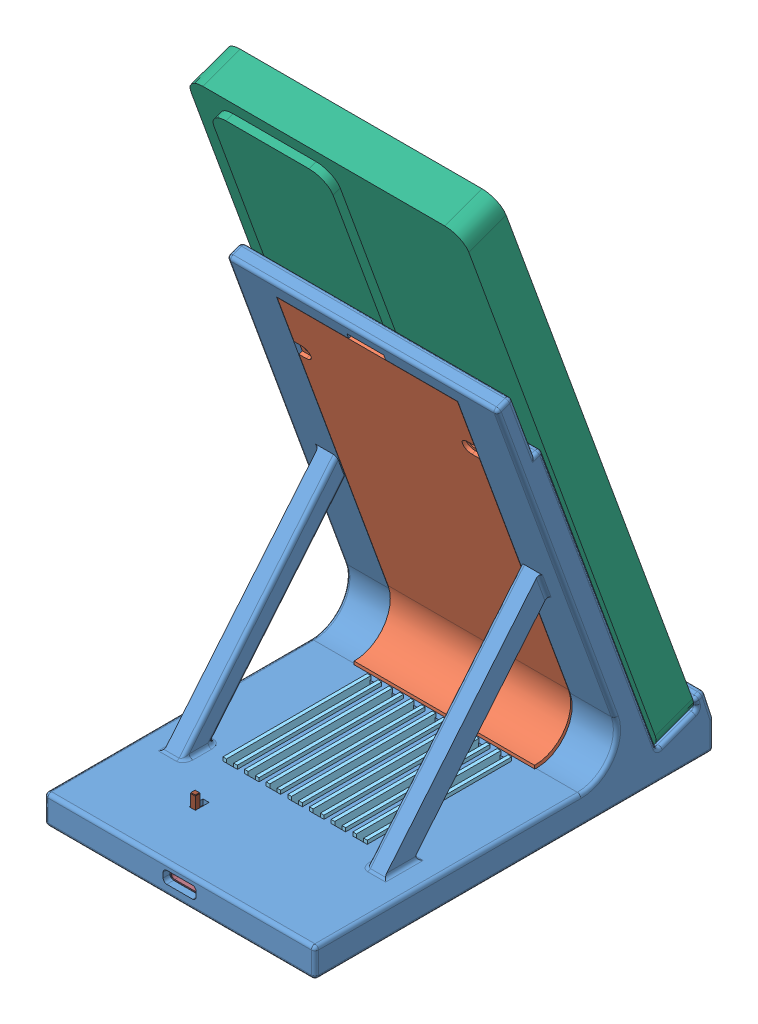
SolidWorks assembly IP支架装配体_倒, configuration 默认. Lengths in mm.
Overall size (77 163.11 111.5).
38 component instances, 18 part files, 24 mates.
Components (placement in the parent):
- IP支架_倒-1: IP支架_倒 [默认] at (-67.6479 -61.183 124.564) size (75 112.62 110.5)
- 支架零件-1: 支架零件 [默认] at (-67.6479 -57.3497 135.0646) x (0 0 -1) z (1 0 0) size (34.38 102 50)
- IP手机-1: IP手机 [默认] at (-19.3867 44.2514 95.8225) x (1 0 0) z (0 0.939693 0.34202) size (76 12 151) (hidden)
- 充电线圈-1: 充电线圈 [默认] at (-67.6479 22.7276 116.3435) x (1 0 0) z (0 -0.939693 -0.34202) size (43 1.52 55.03)
- 充电零件板-1: 充电零件板 [默认] at (-67.7479 -57.183 127.464) x (1 0 0) z (0 0 -1) size (21 2 28)
- 散热器-1: 散热器 [默认] at (-67.7479 -57.183 127.464) size (40 5 40)
- P60手机-1: P60手机 [默认] at (-67.6479 22.4622 112.0966) x (-1 0 0) z (0 0.34202 -0.939693) size (77 161 13.1)
- Led5mmRojo_.step-1: Led5mmRojo_.step [默认] at (-67.6479 -56.683 93.564) x (0 0 -1) z (0.800625 -0.599165 0) size (25.5 5.8 5.4)
- 底板_倒-1: 底板_倒 [默认] at (-83.0896 -61.183 121.7495) x (0 0 -1) z (1 0 0) size (101.9 5.8 64.8) (hidden)
- TypeC电路板_倒.step-1: TypeC电路板_倒.step [默认] at (-45.6508 -59.6431 180.9032) x (0 0 -1) z (0 1 0) size (30 34.97 18.44)
  - cTDU-R1.step-1: cTDU-R1.step [默认] at (26.2129 13.5382 1.2) x (0 1 0) z (0 0 1) size (2 1.3 0.61)
    - R0805.step-1: R0805.step [默认] at origin size (2 1.3 0.61)
      - COMPOUND.step-1: COMPOUND.step [默认] at origin size (2 1.3 0.61)
  - cTDU-U4.step-1: cTDU-U4.step [默认] at (18.386 14.645 1.2) size (4.1 4.3 1.61)
    - SOT-89-3_L4.5-W2.5-P1.50-LS4.2-BR.step-1: SOT-89-3_L4.5-W2.5-P1.50-LS4.2-BR.step [默认] at origin size (4.1 4.3 1.61)
      - SOLID.step-1: SOLID.step [默认] at origin size (4.1 4.3 1.61)
  - cTDU-C1.step-1: cTDU-C1.step [默认] at (18.2118 28.8799 1.2) size (3.2 2.52 0.9)
    - C1210.step-1: C1210.step [默认] at origin size (3.2 2.52 0.9)
      - SOLID-0.step-1: SOLID-0.step [默认] at origin size (3.2 2.52 0.9)
  - cTDU-H2.step-1: cTDU-H2.step [默认] at (29.8197 31.3945 0) x (0 1 0) z (0 0 -1) size (2.55 2.54 11.5)
    - HDR-TH_1P-P2.54-V-M.step-1: HDR-TH_1P-P2.54-V-M.step [默认] at origin size (2.55 2.54 11.5)
      - SOLID-1.step-1: SOLID-1.step [默认] at origin size (2.55 2.54 11.5) (hidden)
  - cTDU-H1.step-1: cTDU-H1.step [默认] at (29.8451 12.5476 0) x (0 -1 0) z (0 0 -1) size (2.55 2.54 11.5)
    - HDR-TH_1P-P2.54-V-M.step-1: HDR-TH_1P-P2.54-V-M.step [默认] at origin size (2.55 2.54 11.5)
      - SOLID-1.step-1: SOLID-1.step [默认] at origin size (2.55 2.54 11.5) (hidden)
  - cTDU-U2.step-1: cTDU-U2.step [默认] at (19.685 34.9251 1.2) size (8.51 3.81 11.5)
    - SW-TH_DEALON_SS-12D01-GX.step-1: SW-TH_DEALON_SS-12D01-GX.step [默认] at origin size (8.51 3.81 11.5)
      - COMPOUND-2.step-1: COMPOUND-2.step [默认] at origin size (8.51 3.81 11.5)
  - cTDU-U3.step-1: cTDU-U3.step [默认] at (29.8451 21.997 0) x (0 1 0) z (0 0 -1) size (12.71 2.54 11.54)
    - HDR-TH_5P-P2.54-V-M.step-1: HDR-TH_5P-P2.54-V-M.step [默认] at origin size (12.71 2.54 11.54)
      - SOLID-3.step-1: SOLID-3.step [默认] at origin size (12.71 2.54 11.54) (hidden)
  - cTDU-C2.step-1: cTDU-C2.step [默认] at (22.4282 13.843 1.2) x (0 1 0) z (0 0 1) size (1.6 0.8 0.8)
    - C0603.step-1: C0603.step [默认] at origin size (1.6 0.8 0.8)
      - SOLID-4.step-1: SOLID-4.step [默认] at origin size (1.6 0.8 0.8)
  - cTDU-USB1.step-1: cTDU-USB1.step [默认] at (8.1992 21.9972 1.2) x (0 -1 0) z (0 0 1) size (8.95 7.58 4.16)
    - USB-C-SMD_TYPE-C-6PIN-2MD-073.step-1: USB-C-SMD_TYPE-C-6PIN-2MD-073.step [默认] at origin size (8.95 7.58 4.16)
      - COMPOUND-5.step-1: COMPOUND-5.step [默认] at origin size (8.95 7.58 4.16)
  - Board.step-1: Board.step [默认] at origin size (29.97 34.97 1.2)
Mates (geometry in assembly coordinates):
- 重合8: coincident anti-aligned: plane of 支架零件-1 through (-67.6479 22.2146 117.753) normal (0 0.34202 -0.939693); plane of 充电线圈-1 through (-67.6479 22.2146 117.753) normal (0 -0.34202 0.939693)
- 同心1: concentric aligned: cylinder of 支架零件-1 through (-67.6479 22.2146 117.753) axis (0 0.34202 -0.939693) radius 22; cylinder of 充电线圈-1 through (-67.6479 22.2146 117.753) axis (0 0.34202 -0.939693) radius 21.5
- 重合15: coincident aligned: plane of 支架零件-1 through (-67.6479 -57.3497 135.0646) normal (1 0 0); plane of 充电线圈-1 through (-67.6479 22.7276 116.3435) normal (1 0 0)
- 重合43: coincident anti-aligned: plane of 充电零件板-1 through (-69.7479 -57.183 121.839) normal (0 1 0); plane of 散热器-1 through (-67.7479 -57.183 127.464) normal (0 -1 0)
- 宽度9: width aligned: plane of 散热器-1 through (-87.7479 -55.183 107.464) normal (-1 0 0); plane of 充电零件板-1 through (-47.7479 -55.183 107.464) normal (1 0 0); plane of 散热器-1 through (-78.2479 -59.183 138.464) normal (-1 0 0); plane of 充电零件板-1 through (-57.2479 -59.183 138.464) normal (1 0 0)
- 宽度10: width anti-aligned: plane of IP支架_倒-1 through (-92.7479 -43.183 105.869) normal (1 0 0); plane of 支架零件-1 through (-42.5479 -43.183 105.869) normal (-1 0 0); plane of IP支架_倒-1 through (-92.6479 -42.3 106.1904) normal (-1 0 0); plane of 支架零件-1 through (-42.6479 -42.3 106.1904) normal (1 0 0)
- 距离1: distance = 0.1 mm anti-aligned: plane of 支架零件-1 through (-42.6479 45.6723 127.5679) normal (0 0.939693 0.34202); plane of IP支架_倒-1 through (-92.7479 -162620.1292 447048.4771) normal (0 -0.939693 -0.34202)
- 重合45: coincident aligned: plane of IP支架_倒-1 through (84.5237 -53.183 91.5875) normal (0 -0.34202 0.939693); plane of 支架零件-1 through (-42.6479 -38.8798 96.7935) normal (0 -0.34202 0.939693)
- 重合47: coincident anti-aligned: plane of IP支架_倒-1 through (84.5237 52.4405 123.0078) normal (0 0.34202 -0.939693); plane of P60手机-1 through (-67.6479 22.4622 112.0966) normal (0 -0.34202 0.939693)
- 宽度11: width aligned: plane of P60手机-1 through (-106.1479 101.8697 129.2926) normal (-1 0 0); plane of IP支架_倒-1 through (-29.1479 101.8697 129.2926) normal (1 0 0); plane of P60手机-1 through (-105.1479 -53.183 179.564) normal (-1 0 0); plane of IP支架_倒-1 through (-30.1479 -53.183 179.564) normal (1 0 0)
- 重合48: coincident anti-aligned: plane of IP支架_倒-1 through (-67.6479 -55.183 124.564) normal (0 -1 0); plane of 散热器-1 through (-67.7479 -55.183 127.464) normal (0 1 0)
- 宽度12: width anti-aligned: plane of 散热器-1 through (-47.7479 -55.183 107.464) normal (1 0 0); plane of IP支架_倒-1 through (-87.7479 -55.183 107.464) normal (-1 0 0); plane of 散热器-1 through (-47.7479 -61.184 107.664) normal (-1 0 0); plane of IP支架_倒-1 through (-87.7479 -61.184 107.664) normal (1 0 0)
- 重合49: coincident anti-aligned: plane of IP支架_倒-1 through (-81.7479 -61.184 147.464) normal (0 0 -1); plane of 散热器-1 through (-87.7479 -55.183 147.464) normal (0 0 1)
- 宽度13: width aligned: plane of 散热器-1 through (-87.7479 -55.183 107.464) normal (0 0 -1); plane of 充电零件板-1 through (-87.7479 -55.183 147.464) normal (0 0 1); plane of 散热器-1 through (-71.2479 -59.183 113.464) normal (0 0 -1); plane of 充电零件板-1 through (-75.7479 -59.183 141.464) normal (0 0 1)
- 平行1: parallel aligned: plane of IP支架_倒-1 through (-67.6479 -55.183 124.564) normal (0 -1 0); plane of TypeC电路板_倒.step-1/Board.step-1 through (-67.6479 -59.6431 161.3502) normal (0 -1 0)
- 平行2: parallel aligned: plane of IP支架_倒-1 through (-105.1479 -53.183 179.564) normal (0 0 1); plane of TypeC电路板_倒.step-1/Board.step-1 through (-61.6606 -59.6431 177.6663) normal (0 0 1)
- 宽度14: width anti-aligned: plane of TypeC电路板_倒.step-1/Board.step-1 through (-73.6352 -59.6431 177.6663) normal (-1 0 0); plane of IP支架_倒-1 through (-61.6606 -59.6431 170.179) normal (1 0 0); plane of TypeC电路板_倒.step-1/Board.step-1 through (-73.7352 -61.184 291668.814) normal (1 0 0); plane of IP支架_倒-1 through (-61.5606 -61.184 291668.814) normal (-1 0 0)
- 重合51: coincident anti-aligned: plane of IP支架_倒-1 through (-400067.6479 -61.184 177.6663) normal (0 0 -1); plane of TypeC电路板_倒.step-1/Board.step-1 through (-61.6606 -59.6431 177.6663) normal (0 0 1)
- 重合53: coincident anti-aligned: plane of IP支架_倒-1 through (-67.6479 -55.183 124.564) normal (0 -1 0); plane of TypeC电路板_倒.step-1/cTDU-USB1.step-1/USB-C-SMD_TYPE-C-6PIN-2MD-073.step-1/COMPOUND-5.step-1 through (-70.868 -55.183 170.364) normal (0 1 0)
- 重合54: coincident aligned: plane of IP支架_倒-1 through (-67.6479 -61.183 124.564) normal (0 -1 0); plane of 底板_倒-1 through (-83.0896 -61.183 121.7495) normal (0 -1 0)
- 宽度15: width anti-aligned: plane of IP支架_倒-1 through (-35.1479 -61.184 291668.814) normal (-1 0 0); plane of 底板_倒-1 through (-100.1479 -61.184 291668.814) normal (1 0 0); plane of IP支架_倒-1 through (-35.2479 -59.683 173.464) normal (1 0 0); plane of 底板_倒-1 through (-100.0479 -59.683 173.464) normal (-1 0 0)
- 宽度16: width aligned: plane of 底板_倒-1 through (-100.0479 -59.683 75.664) normal (0 0 -1); plane of IP支架_倒-1 through (-61.6606 -59.683 173.464) normal (0 0 1); plane of 底板_倒-1 through (-400067.6479 -61.184 173.564) normal (0 0 -1); plane of IP支架_倒-1 through (-400067.6479 -61.184 75.564) normal (0 0 1)
- 同心2: concentric: cylinder of IP支架_倒-1 through (-67.6479 -56.683 82.9179) axis (0 0 -1) radius 2.6; cylinder of Led5mmRojo_.step-1 through (-67.6479 -56.683 80.9686) axis (0 0 -1) radius 2.5
- 重合55: coincident anti-aligned: plane of IP支架_倒-1 through (-400067.6479 -61.184 75.564) normal (0 0 1); plane of Led5mmRojo_.step-1 through (-67.4878 -56.8029 80.9686) normal (0 0 -1)
